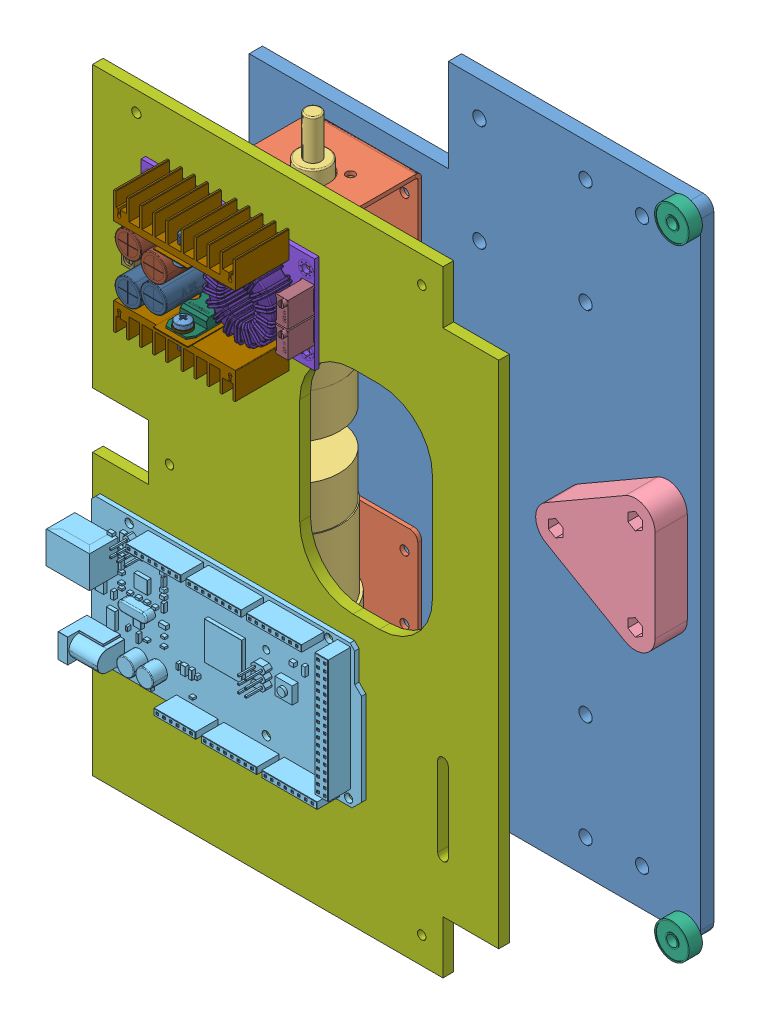
SolidWorks assembly robot_sghyr, configuration Default. Lengths in mm.
Overall size (182.75 247 92.25).
86 component instances, 28 part files, 23 mates.
Components (placement in the parent):
- base_robot_sghyr-1: base_robot_sghyr [Default] at (64.264 97.0127 214.7631) size (170 240 5)
- 37 mm DC Geared Motor Mounting Bracket-1: 37 mm DC Geared Motor Mounting Bracket [Default] at (24.264 176.3252 247.7631) x (0 -1 0) z (-1 0 0) size (41 48 40)
- pololu-37D-encoder-1: pololu-37D-encoder [Default] at (24.264 150.5252 247.7631) x (0 0 -1) z (0 1 0) size (36.8 36.8 92.61)
- Robot2015_support bille porteuse-1: Robot2015_support bille porteuse [Défaut] at (126.764 97.0127 219.7631) x (-0.866025 -0.5 0) z (-0.5 0.866025 0) size (49.64 16.2 45)
- 37 mm DC Geared Motor Mounting Bracket-3: 37 mm DC Geared Motor Mounting Bracket [Default] at (24.264 17.7002 247.7631) x (0 1 0) z (1 0 0) size (41 48 40)
- pololu-37D-encoder-4: pololu-37D-encoder [Default] at (24.264 43.5002 247.7631) x (0 0 -1) z (0 -1 0) size (36.8 36.8 92.61)
- Arduino Mega 2560.step-1: Arduino Mega 2560.step [Default] at (36.414 47.7208 285.4141) x (-1 0 0) z (0 0 -1) size (107.95 53.42 12.95)
- Roulement_d3xd10xe4-1: Roulement_d3xd10xe4 [Défaut] at (146.264 -19.9873 225.0631) x (0 0 1) z (-1 0 0) size (5 13 13)
- etage electronique-1: etage electronique [Default] at (64.264 97.0127 279.7631) x (0 -1 0) z (0 0 1) size (232 153 4)
- XL4016E1 8A Buck Converter.STEP-1: XL4016E1 8A Buck Converter.STEP [Default] at (36.914 174.7627 283.7631) x (1 0 0) z (0 -1 0) size (65.3 28.6 46.4)
  - 8A Buck Converter PCB.STEP-1: 8A Buck Converter PCB.STEP [Default] at origin size (65.3 1.67 36.5)
  - Heat Exchanger.STEP-1: Heat Exchanger.STEP [Default] at (0 1.65 23.2) size (46 25.1 10.55)
  - Heat Exchanger.STEP-2: Heat Exchanger.STEP [Default] at (0 1.65 -23.2) x (-1 0 0) z (0 0 -1) size (46 25.1 10.55)
  - LargeGreen1000uF 35V Electrolytic Capacitor.STEP-1: LargeGreen1000uF 35V Electrolytic Capacitor.STEP [Default] at (-17.6782 1.65 7.8366) x (0 0 -1) z (1 0 0) size (9.9 26.01 9.9)
  - LargeGreen1000uF 35V Electrolytic Capacitor.STEP-2: LargeGreen1000uF 35V Electrolytic Capacitor.STEP [Default] at (-8.0317 1.65 5.0694) x (0 0 -1) z (1 0 0) size (9.9 26.01 9.9)
  - LargeGreen470uF 35V Electrolytic Capacitor.STEP-1: LargeGreen470uF 35V Electrolytic Capacitor.STEP [Default] at (-17.6617 1.65 -7.7514) x (0 0 1) z (-1 0 0) size (9.9 26.01 9.9)
  - LargeGreen470uF 35V Electrolytic Capacitor.STEP-2: LargeGreen470uF 35V Electrolytic Capacitor.STEP [Default] at (-7.9869 1.65 -5.0151) x (0 0 1) z (-1 0 0) size (9.9 26.01 9.9)
  - Screw Terminal x2.STEP-1: Screw Terminal x2.STEP [Default] at (-9.5 0 12.7839) x (-1 0 0) z (0 0 -1) size (7.95 12.9 10)
  - Screw Terminal x2.STEP-2: Screw Terminal x2.STEP [Default] at (-9.5 0 2.7839) x (-1 0 0) z (0 0 -1) size (7.95 12.9 10)
  - TrimmerW103.STEP-1: TrimmerW103.STEP [Default] at (32.65 6.9 -4.9563) x (0 0 1) z (-1 0 0) size (9.5 15.15 4.8)
  - TrimmerW103.STEP-2: TrimmerW103.STEP [Default] at (32.65 6.9 5.0581) x (0 0 1) z (-1 0 0) size (9.5 15.15 4.8)
  - whiteLEDShortLeed.STEP-1: whiteLEDShortLeed.STEP [Default] at (-13.9989 2.65 -0.1564) x (-1 0 0) z (0 0 -1) size (3.4 13.35 3.4)
  - Schottky Diode 20A 45V STPS2045CT.STEP-1: Schottky Diode 20A 45V STPS2045CT.STEP [Default] at (-0.0419 13.7002 12.65) x (-0.999962 0.008727 0) z (-0.008727 -0.999962 0) size (10.22 3.95 22.6)
  - XL4016E1 8A Voltage Regulator.STEP-1: XL4016E1 8A Voltage Regulator.STEP [Default] at (0 13.7 -12.65) x (1 0 0) z (0 -1 0) size (10.22 3.95 22.6)
  - Coil for Convertor.STEP-1: Coil for Convertor.STEP [Default] at (14.3115 2.9157 0.0112) size (27.99 14.39 26.86)
  - Small Plastic Washer.STEP-1: Small Plastic Washer.STEP [Default] at (0 18.5 -11.95) x (1 0 0) z (0 -1 0) size (6.1 1 6.1)
  - Small Plastic Washer.STEP-2: Small Plastic Washer.STEP [Default] at (0 18.5 10.95) x (1 0 0) z (0 -1 0) size (6.1 1 6.1)
  - pan head cross recess screw_iso_ISO 7045 - M3 x 8 - Z - 8S.STEP-1: pan head cross recess screw_iso_ISO 7045 - M3 x 8 - Z - 8S.STEP [Default] at (0 18.5 -8.55) x (0 0 -1) z (0.923728 0.383049 0) size (10.36 5.6 5.6)
  - pan head cross recess screw_iso_ISO 7045 - M3 x 8 - Z - 8S.STEP-2: pan head cross recess screw_iso_ISO 7045 - M3 x 8 - Z - 8S.STEP [Default] at (0 18.5 8.55) x (0 0 1) z (-1 0 0) size (10.36 5.6 5.6)
  - 1.7mmSmdCeramicCapacitorbrown.STEP-1: 1.7mmSmdCeramicCapacitorbrown.STEP [Default] at (2.849 0.0574 -8.3522) x (-1 0 0) z (0 0 1) size (2.02 0.49 1.04)
  - smdChip8pin.STEP-1: smdChip8pin.STEP [Default] at (19.9049 -0.725 7.6791) x (1 0 0) z (0 0 -1) size (7.3 1.22 4.5)
  - tinyVoltageRegulator.STEP-1: tinyVoltageRegulator.STEP [Default] at (13.3487 0 4.1964) x (-1 0 0) z (0 0 1) size (2.75 0.7 2.1)
  - tinyVoltageRegulator.STEP-2: tinyVoltageRegulator.STEP [Default] at (20.3011 0 11.2685) x (0.999962 0 0.008727) z (0.008727 0 -0.999962) size (2.75 0.7 2.1)
  - TinyVoltageRegulatorAMS1112.STEP-1: TinyVoltageRegulatorAMS1112.STEP [Default] at (15.0739 0.203 -4.8321) x (0 0 -1) z (-1 0 0) size (4.07 1.22 4.96)
  - tinySMDResistor222.STEP-1: tinySMDResistor222.STEP [Default] at (21.8501 0.1177 -6.1765) x (0 0 -1) z (-1 0 0) size (1.52 0.38 0.79)
  - tinySMDResistor.STEP-1: tinySMDResistor.STEP [Default] at (19.9225 0.1177 -6.1853) x (0 0 -1) z (-1 0 0) size (1.52 0.37 0.79)
  - 1.7mmSmdCeramicCapacitorbrown.STEP-2: 1.7mmSmdCeramicCapacitorbrown.STEP [Default] at (24.1073 0.0574 -6.3061) x (0 0 -1) z (-1 0 0) size (2.02 0.49 1.04)
  - 1.7mmSmdCeramicCapacitorbrown.STEP-3: 1.7mmSmdCeramicCapacitorbrown.STEP [Default] at (16.3262 0.0574 0.9562) x (0 0 -1) z (-1 0 0) size (2.02 0.49 1.04)
  - 1.7mmSmdCeramicCapacitorbrown.STEP-4: 1.7mmSmdCeramicCapacitorbrown.STEP [Default] at (18.1093 0.0574 0.9562) x (0 0 -1) z (-1 0 0) size (2.02 0.49 1.04)
  - tinySMDResistor.STEP-2: tinySMDResistor.STEP [Default] at (19.9874 0.1177 1.1419) x (0 0 -1) z (-1 0 0) size (1.52 0.37 0.79)
  - tinySMDResistor.STEP-3: tinySMDResistor.STEP [Default] at (21.6733 0.1177 1.1419) x (0 0 -1) z (-1 0 0) size (1.52 0.37 0.79)
  - tinySMDResistor.STEP-4: tinySMDResistor.STEP [Default] at (23.3916 0.1177 1.1419) x (0 0 -1) z (-1 0 0) size (1.52 0.37 0.79)
  - 1.7mmSmdCeramicCapacitorbrown.STEP-5: 1.7mmSmdCeramicCapacitorbrown.STEP [Default] at (25.4211 0.0574 4.0139) x (0 0 -1) z (-1 0 0) size (2.02 0.49 1.04)
  - 1.7mmSmdCeramicCapacitorbrown.STEP-6: 1.7mmSmdCeramicCapacitorbrown.STEP [Default] at (27.3088 0.0574 4.0139) x (0 0 -1) z (-1 0 0) size (2.02 0.49 1.04)
  - 1.7mmSmdCeramicCapacitorbrown.STEP-7: 1.7mmSmdCeramicCapacitorbrown.STEP [Default] at (23.1777 0.0574 11.1322) x (0 0 -1) z (-1 0 0) size (2.02 0.49 1.04)
  - 1.7mmSmdCeramicCapacitorbrown.STEP-8: 1.7mmSmdCeramicCapacitorbrown.STEP [Default] at (20.6839 0.0574 9.112) x (-0.999962 0 -0.008727) z (-0.008727 0 0.999962) size (2.02 0.49 1.04)
  - tinySMDResistor.STEP-5: tinySMDResistor.STEP [Default] at (17.7351 0.1177 11.3427) x (0 0 -1) z (-1 0 0) size (1.52 0.37 0.79)
  - tinySMDResistor.STEP-6: tinySMDResistor.STEP [Default] at (16.0827 0.1177 11.3427) x (0 0 -1) z (-1 0 0) size (1.52 0.37 0.79)
  - tinySMDResistor.STEP-7: tinySMDResistor.STEP [Default] at (16.906 0.1177 9.0199) x (-0.999962 0 -0.008727) z (-0.008727 0 0.999962) size (1.52 0.37 0.79)
  - tinySMDResistor.STEP-8: tinySMDResistor.STEP [Default] at (25.3907 0.1177 9.8144) x (-0.999962 0 -0.008727) z (-0.008727 0 0.999962) size (1.52 0.37 0.79)
  - R010 Resistor SMD.STEP-1: R010 Resistor SMD.STEP [Default] at (-19.919 0 5.2469) x (0 0 -1) z (-1 0 0) size (6.7 0.52 3.1)
  - solder.STEP-1: solder.STEP [Default] at (-27.65 0 -7.4411) x (-0.837169 0 -0.546944) z (-0.546944 0 0.837169) size (1.17 0.65 1.17)
  - solder.STEP-2: solder.STEP [Default] at (-27.65 0 -2.711) x (-0.837169 0 -0.546944) z (-0.546944 0 0.837169) size (1.17 0.65 1.17)
  - solder.STEP-3: solder.STEP [Default] at (-27.65 0 2.537) x (-0.837169 0 -0.546944) z (-0.546944 0 0.837169) size (1.17 0.65 1.17)
  - solder.STEP-4: solder.STEP [Default] at (-27.65 0 7.3016) x (-0.837169 0 -0.546944) z (-0.546944 0 0.837169) size (1.17 0.65 1.17)
  - solder1.8.STEP-1: solder1.8.STEP [Default] at (-20.8987 0 -15.5519) x (-0.837169 0 -0.546944) z (-0.546944 0 0.837169) size (1.8 0.65 1.8)
  - solder1.8.STEP-2: solder1.8.STEP [Default] at (20.8325 0 -15.5519) x (-0.837169 0 -0.546944) z (-0.546944 0 0.837169) size (1.8 0.65 1.8)
  - solder1.8.STEP-3: solder1.8.STEP [Default] at (20.8325 0 15.5391) x (-0.837169 0 -0.546944) z (-0.546944 0 0.837169) size (1.8 0.65 1.8)
  - solder1.8.STEP-4: solder1.8.STEP [Default] at (-20.8987 0 15.5391) x (-0.837169 0 -0.546944) z (-0.546944 0 0.837169) size (1.8 0.65 1.8)
  - solder.STEP-5: solder.STEP [Default] at (30.4698 0 7.6228) x (-0.837169 0 -0.546944) z (-0.546944 0 0.837169) size (1.17 0.65 1.17)
  - solder.STEP-6: solder.STEP [Default] at (30.4698 0 2.537) x (-0.837169 0 -0.546944) z (-0.546944 0 0.837169) size (1.17 0.65 1.17)
  - solder.STEP-7: solder.STEP [Default] at (30.4698 0 -2.454) x (-0.837169 0 -0.546944) z (-0.546944 0 0.837169) size (1.17 0.65 1.17)
  - solder.STEP-8: solder.STEP [Default] at (30.4698 0 -7.4732) x (-0.837169 0 -0.546944) z (-0.546944 0 0.837169) size (1.17 0.65 1.17)
  - solder.STEP-9: solder.STEP [Default] at (30.4698 0 -4.9355) x (-0.837169 0 -0.546944) z (-0.546944 0 0.837169) size (1.17 0.65 1.17)
  - solder.STEP-10: solder.STEP [Default] at (30.4698 0 5.0529) x (-0.837169 0 -0.546944) z (-0.546944 0 0.837169) size (1.17 0.65 1.17)
  - solder1.8.STEP-5: solder1.8.STEP [Default] at (1.0959 0 2.1506) x (-0.837169 0 -0.546944) z (-0.546944 0 0.837169) size (1.8 0.65 1.8)
  - solder1.8.STEP-6: solder1.8.STEP [Default] at (8.9457 0 2.3519) x (-0.837169 0 -0.546944) z (-0.546944 0 0.837169) size (1.8 0.65 1.8)
  - solder.STEP-11: solder.STEP [Default] at (-3.9931 0 -10.2017) x (-0.837169 0 -0.546944) z (-0.546944 0 0.837169) size (1.17 0.65 1.17)
  - solder.STEP-12: solder.STEP [Default] at (-1.9931 0 -10.2017) x (-0.837169 0 -0.546944) z (-0.546944 0 0.837169) size (1.17 0.65 1.17)
  - solder.STEP-13: solder.STEP [Default] at (0.0069 0 -10.2017) x (-0.837169 0 -0.546944) z (-0.546944 0 0.837169) size (1.17 0.65 1.17)
  - solder.STEP-14: solder.STEP [Default] at (2.0069 0 -10.2017) x (-0.837169 0 -0.546944) z (-0.546944 0 0.837169) size (1.17 0.65 1.17)
  - solder.STEP-15: solder.STEP [Default] at (4.0069 0 -10.2017) x (-0.837169 0 -0.546944) z (-0.546944 0 0.837169) size (1.17 0.65 1.17)
  - solder.STEP-16: solder.STEP [Default] at (-2.7433 0 10.0764) x (-0.873283 0 -0.487214) z (-0.487214 0 0.873283) size (1.17 0.65 1.17)
  - solder.STEP-17: solder.STEP [Default] at (-0.2033 0 10.0764) x (-0.873283 0 -0.487214) z (-0.487214 0 0.873283) size (1.17 0.65 1.17)
  - solder.STEP-18: solder.STEP [Default] at (2.3367 0 10.0764) x (-0.873283 0 -0.487214) z (-0.487214 0 0.873283) size (1.17 0.65 1.17)
  - solder.STEP-19: solder.STEP [Default] at (-8.0296 0 7.8897) x (-0.873283 0 -0.487214) z (-0.487214 0 0.873283) size (1.17 0.65 1.17)
  - solder.STEP-20: solder.STEP [Default] at (-8.0296 0 2.259) x (-0.873283 0 -0.487214) z (-0.487214 0 0.873283) size (1.17 0.65 1.17)
  - solder.STEP-21: solder.STEP [Default] at (-8.0296 0 -2.2341) x (-0.873283 0 -0.487214) z (-0.487214 0 0.873283) size (1.17 0.65 1.17)
  - solder.STEP-22: solder.STEP [Default] at (-8.0296 0 -7.8634) x (-0.873283 0 -0.487214) z (-0.487214 0 0.873283) size (1.17 0.65 1.17)
  - solder.STEP-23: solder.STEP [Default] at (-17.6872 0 -10.549) x (-0.873283 0 -0.487214) z (-0.487214 0 0.873283) size (1.17 0.65 1.17)
  - solder.STEP-24: solder.STEP [Default] at (-17.6872 0 -4.9388) x (-0.873283 0 -0.487214) z (-0.487214 0 0.873283) size (1.17 0.65 1.17)
  - solder.STEP-25: solder.STEP [Default] at (-17.6872 0 10.6333) x (-0.873283 0 -0.487214) z (-0.487214 0 0.873283) size (1.17 0.65 1.17)
  - solder.STEP-26: solder.STEP [Default] at (-17.6872 0 5.0231) x (-0.873283 0 -0.487214) z (-0.487214 0 0.873283) size (1.17 0.65 1.17)
  - solder.STEP-27: solder.STEP [Default] at (-15.2798 0 -0.193) x (-0.873283 0 -0.487214) z (-0.487214 0 0.873283) size (1.17 0.65 1.17)
  - solder.STEP-28: solder.STEP [Default] at (-12.7921 0 -0.193) x (-0.873283 0 -0.487214) z (-0.487214 0 0.873283) size (1.17 0.65 1.17)
- Roulement_d3xd10xe4-3: Roulement_d3xd10xe4 [Défaut] at (146.264 214.0127 225.0631) x (0 0 1) z (1 0 0) size (5 13 13)
Mates (geometry in assembly coordinates):
- Coincident2: coincident anti-aligned: plane of 37 mm DC Geared Motor Mounting Bracket-1 through (24.264 174.8252 247.7631) normal (0 -1 0); plane of pololu-37D-encoder-1 through (24.264 174.8252 247.7631) normal (0 1 0)
- Concentric8: concentric anti-aligned: cylinder of 37 mm DC Geared Motor Mounting Bracket-1 through (24.264 135.3252 240.7631) axis (0 1 0) radius 6.5; cylinder of pololu-37D-encoder-1 through (24.264 181.3252 240.7631) axis (0 -1 0) radius 6
- Concentric10: concentric aligned: cylinder of 37 mm DC Geared Motor Mounting Bracket-1 through (32.014 176.3252 261.1865) axis (0 1 0) radius 1.6; cylinder of pololu-37D-encoder-1 through (32.014 174.8252 261.1865) axis (0 1 0) radius 1.5
- Coincident4: coincident anti-aligned: plane of base_robot_sghyr-1 through (64.264 97.0127 219.7631) normal (0 0 1); plane of 37 mm DC Geared Motor Mounting Bracket-1 through (4.264 174.8252 219.7631) normal (0 0 -1)
- Parallel4: parallel aligned: plane of base_robot_sghyr-1 through (-20.736 217.0127 219.7631) normal (0 1 0); plane of 37 mm DC Geared Motor Mounting Bracket-1 through (24.264 176.3252 247.7631) normal (0 1 0)
- Coincident14: coincident anti-aligned: plane of 37 mm DC Geared Motor Mounting Bracket-3 through (24.264 19.2002 247.7631) normal (0 1 0); plane of pololu-37D-encoder-4 through (24.264 19.2002 247.7631) normal (0 -1 0)
- Parallel9: parallel aligned: plane of base_robot_sghyr-1 through (149.264 217.0127 219.7631) normal (1 0 0); plane of Robot2015_support bille porteuse-1 through (144.264 79.6922 231.8631) normal (1 0 0)
- Coincident17: coincident anti-aligned: plane of base_robot_sghyr-1 through (64.264 97.0127 219.7631) normal (0 0 1); plane of Robot2015_support bille porteuse-1 through (136.764 79.6922 219.7631) normal (0 0 -1)
- Distance2: distance = 25 mm aligned: plane of 37 mm DC Geared Motor Mounting Bracket-1 through (4.264 176.3252 247.7631) normal (-1 0 0); plane of base_robot_sghyr-1 through (-20.736 217.0127 219.7631) normal (-1 0 0)
- Parallel11: parallel anti-aligned: plane of base_robot_sghyr-1 through (64.264 97.0127 219.7631) normal (0 0 1); plane of Roulement_d3xd10xe4-1 through (146.264 -17.4873 222.5631) normal (0 0 -1)
- Distance3: distance = 3 mm: cylinder of Roulement_d3xd10xe4-1 through (146.264 -19.9873 222.5631) axis (0 0 -1) radius 2; plane of base_robot_sghyr-1 through (-20.736 -22.9873 219.7631) normal (0 -1 0)
- Distance4: distance = 3 mm: cylinder of Roulement_d3xd10xe4-1 through (146.264 -19.9873 222.5631) axis (0 0 -1) radius 2; plane of base_robot_sghyr-1 through (149.264 217.0127 219.7631) normal (1 0 0)
- Distance5: distance = 5 mm aligned: plane of Robot2015_support bille porteuse-1 through (144.264 79.6922 231.8631) normal (1 0 0); plane of base_robot_sghyr-1 through (149.264 217.0127 219.7631) normal (1 0 0)
- Parallel13: parallel aligned: plane of base_robot_sghyr-1 through (64.264 97.0127 219.7631) normal (0 0 1); plane of etage electronique-1 through (64.264 97.0127 283.7631) normal (0 0 1)
- Width2: width anti-aligned: plane of etage electronique-1 through (149.264 -18.9873 283.7631) normal (0 -1 0); plane of base_robot_sghyr-1 through (149.264 213.0127 283.7631) normal (0 1 0); plane of etage electronique-1 through (-20.736 217.0127 219.7631) normal (0 1 0); plane of base_robot_sghyr-1 through (-20.736 -22.9873 219.7631) normal (0 -1 0)
- Coincident32: coincident anti-aligned: plane of Arduino Mega 2560.step-1 through (-14.386 21.0127 283.7631) normal (0 0 -1); plane of etage electronique-1 through (64.264 97.0127 283.7631) normal (0 0 1)
- Coincident57: coincident aligned: plane of base_robot_sghyr-1 through (-20.736 217.0127 219.7631) normal (-1 0 0); plane of Arduino Mega 2560.step-1 through (-20.736 65.1579 296.2091) normal (-1 0 0)
- Concentric20: concentric anti-aligned: cylinder of 37 mm DC Geared Motor Mounting Bracket-3 through (24.264 58.7002 240.7631) axis (0 -1 0) radius 6.5; cylinder of pololu-37D-encoder-4 through (24.264 12.7002 240.7631) axis (0 1 0) radius 6
- Concentric23: concentric aligned: cylinder of 37 mm DC Geared Motor Mounting Bracket-3 through (8.764 17.7002 247.7631) axis (0 -1 0) radius 1.6; cylinder of pololu-37D-encoder-4 through (8.764 19.2002 247.7631) axis (0 -1 0) radius 1.5
- Coincident58: coincident anti-aligned: plane of etage electronique-1 through (64.264 97.0127 283.7631) normal (0 0 1); plane of XL4016E1 8A Buck Converter.STEP-1/8A Buck Converter PCB.STEP-1 through (36.914 174.7627 283.7631) normal (0 0 -1)
- Distance7: distance = 20 mm aligned: plane of XL4016E1 8A Buck Converter.STEP-1/8A Buck Converter PCB.STEP-1 through (4.264 156.5127 285.4131) normal (-1 0 0); plane of etage electronique-1 through (-15.736 213.0127 279.7631) normal (-1 0 0)
- Distance8: distance = 20 mm aligned: plane of XL4016E1 8A Buck Converter.STEP-1/8A Buck Converter PCB.STEP-1 through (4.264 193.0127 285.4131) normal (0 1 0); plane of etage electronique-1 through (149.264 213.0127 283.7631) normal (0 1 0)
- Distance9: distance = 3 mm anti-aligned: plane of base_robot_sghyr-1 through (64.264 97.0127 219.7631) normal (0 0 1); plane of Roulement_d3xd10xe4-1 through (146.264 -13.9873 222.7631) normal (0 0 -1)
